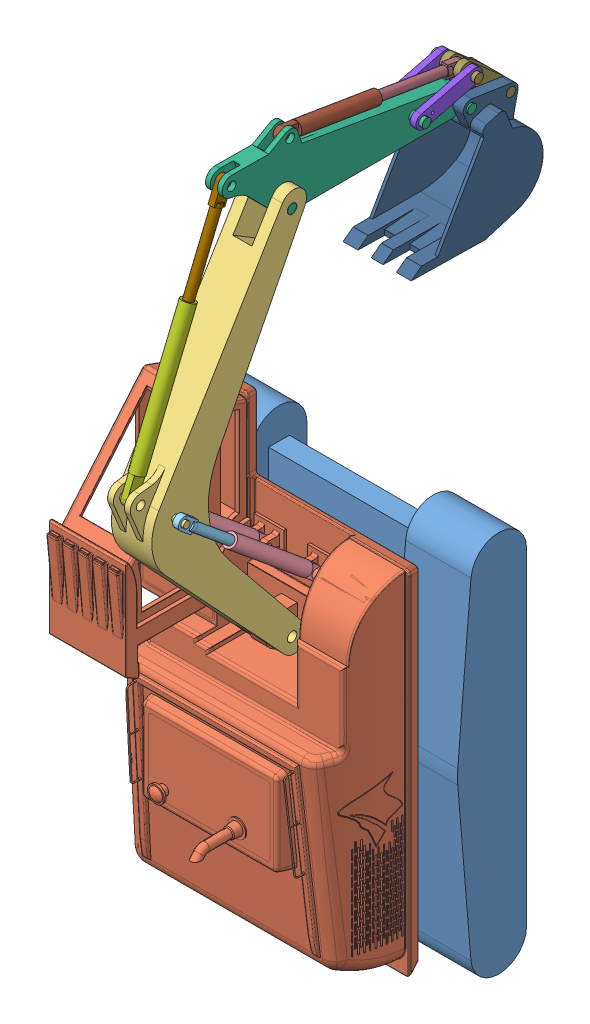
SolidWorks assembly MathScavator9000_flat, configuration Default. Lengths in mm.
Overall size (4800 11820.7 6568.15).
16 component instances, 13 part files, 33 mates.
Components (placement in the parent):
- ExcavatorBase-1: ExcavatorBase [Default] at origin size (4800 6440 1295)
- Chassis_Primary_v2_PART-1: Chassis_Primary_v2_PART [Default] at origin size (3985.01 7287.04 2544.86)
- Boom-2: Boom [Default] at (93.9527 -17.4087 507.5917) size (1080 6775.47 2834.12)
- BoomCyl-2: BoomCyl [Default] at (-446.0473 882.5913 372.5917) x (1 0 0) z (0 0.637047 0.770825) size (223.61 223.61 1900)
- BoomCyl-3: BoomCyl [Default] at (453.9527 882.5913 372.5917) x (1 0 0) z (0 0.637047 0.770825) size (223.61 223.61 1900)
- BoomPiston-2: BoomPiston [Default] at (453.9527 2698.8825 2570.2977) x (1 0 0) z (0 0.637047 0.770825) size (163.61 200 2150)
- BoomPiston-3: BoomPiston [Default] at (-446.0473 2698.8825 2570.2977) x (1 0 0) z (0 0.637047 0.770825) size (163.61 200 2150)
- Stick-1: Stick [Default] at (3.9527 6222.5913 597.5917) size (780 1210.11 4089.97)
- StickCyl-1: StickCyl [Default] at (5.9527 3022.5913 2997.5917) x (1 0 0) z (0 0.924264 -0.381754) size (223.61 223.61 2700)
- StickLink-1: StickLink [Default] at (259.9527 6362.5913 -1642.4083) x (1 0.000056 -0.000224) z (0 0.970634 0.240563) size (100.26 1142.82 240)
- StickLink-2: StickLink [Default] at (-252.0473 6362.5913 -1642.4083) x (1 0.000056 -0.000224) z (0 0.970634 0.240563) size (100.26 1142.82 240)
- StickPiston-1: StickPiston [Default] at (5.9527 6857.8328 1413.4982) x (1 0 0) z (0 0.924264 -0.381754) size (163.61 200 2500)
- Bucket-2: Bucket [Default] at (-1.2473 6213.4488 -2381.9895) size (1148 1959.94 2219.62)
- BucketCyl-2: BucketCyl [Default] at (3.9527 7066.1756 430.7297) x (1 0 0) z (0 -0.162718 -0.986673) size (223.61 223.61 1700)
- BucketLink-2: BucketLink [Default] at (1.9047 6579.7703 -2518.6916) x (1 0.000009 0.00001) z (-0.000013 0.657221 0.753698) size (738.41 251.24 966.87)
- BucketPiston-2: BucketPiston [Default] at (3.9527 6579.7703 -2518.6916) x (1 0 0) z (0 -0.162718 -0.986673) size (163.61 200 1600)
Mates (geometry in assembly coordinates):
- Concentric1: concentric aligned: cylinder of Chassis_Primary_v2_PART-1 through (138.9527 -17.4087 597.5917) axis (1 0 0) radius 80; cylinder of Boom-2 through (343.9527 -17.4087 597.5917) axis (1 0 0) radius 80
- Distance1: distance = 25 mm anti-aligned: plane of Boom-2 through (-156.0473 -1696.3395 2013.4684) normal (1 0 0); plane of Chassis_Primary_v2_PART-1 through (-131.0473 -17.4087 597.5917) normal (-1 0 0)
- Concentric2: concentric aligned: cylinder of Chassis_Primary_v2_PART-1 through (-621.0473 882.5913 372.5917) axis (-1 0 0) radius 40; cylinder of BoomCyl-2 through (-496.0473 882.5913 372.5917) axis (-1 0 0) radius 40
- Distance2: distance = 25 mm anti-aligned: plane of BoomCyl-2 through (-396.0473 959.6738 308.887) normal (1 0 0); plane of Chassis_Primary_v2_PART-1 through (-371.0473 882.5913 372.5917) normal (-1 0 0)
- Distance3: distance = 25 mm anti-aligned: plane of BoomCyl-3 through (403.9527 882.5913 372.5917) normal (-1 0 0); plane of Chassis_Primary_v2_PART-1 through (378.9527 882.5913 372.5917) normal (1 0 0)
- Concentric4: concentric anti-aligned: cylinder of Chassis_Primary_v2_PART-1 through (378.9527 882.5913 372.5917) axis (1 0 0) radius 40; cylinder of BoomCyl-3 through (403.9527 882.5913 372.5917) axis (-1 0 0) radius 40
- Concentric5: concentric anti-aligned: cylinder of Boom-2 through (343.9527 2698.8825 2570.2977) axis (1 0 0) radius 55; cylinder of BoomPiston-2 through (403.9527 2698.8825 2570.2977) axis (-1 0 0) radius 60
- Concentric6: concentric anti-aligned: cylinder of Boom-2 through (-536.0473 2698.8825 2570.2977) axis (1 0 0) radius 55; cylinder of BoomPiston-3 through (-496.0473 2698.8825 2570.2977) axis (-1 0 0) radius 60
- Concentric7: concentric aligned: cylinder of BoomCyl-3 through (453.9527 2029.2762 1760.0764) axis (0 0.637047 0.770825) radius 75; cylinder of BoomPiston-2 through (453.9527 1392.9358 990.1068) axis (0 0.637047 0.770825) radius 72.5
- Concentric8: concentric aligned: cylinder of BoomCyl-2 through (-446.0473 2029.2762 1760.0764) axis (0 0.637047 0.770825) radius 75; cylinder of BoomPiston-3 through (-446.0473 1392.9358 990.1068) axis (0 0.637047 0.770825) radius 72.5
- Concentric9: concentric aligned: cylinder of Boom-2 through (95.9527 3022.5913 2997.5917) axis (-1 0 0) radius 72; cylinder of StickCyl-1 through (-44.0473 3022.5913 2997.5917) axis (-1 0 0) radius 40
- Distance4: distance = 40 mm anti-aligned: plane of StickCyl-1 through (55.9527 3091.9111 2968.9601) normal (1 0 0); plane of Boom-2 through (95.9527 3022.5913 2997.5917) normal (-1 0 0)
- Concentric10: concentric aligned: cylinder of Boom-2 through (163.9527 6222.5913 597.5917) axis (-1 0 0) radius 80; cylinder of Stick-1 through (343.9527 6222.5913 597.5917) axis (-1 0 0) radius 75
- Distance5: distance = 20 mm anti-aligned: plane of Stick-1 through (143.9527 6222.5913 -2282.4083) normal (1 0 0); plane of Boom-2 through (163.9527 3864.7965 -2165.9151) normal (-1 0 0)
- Concentric11: concentric anti-aligned: cylinder of Stick-1 through (143.9527 6857.8328 1413.4982) axis (1 0 0) radius 72; cylinder of StickPiston-1 through (-44.0473 6857.8328 1413.4982) axis (-1 0 0) radius 60
- Concentric12: concentric aligned: cylinder of StickCyl-1 through (5.9527 5425.6772 2005.0303) axis (0 0.924264 -0.381754) radius 75; cylinder of StickPiston-1 through (5.9527 4639.5997 2329.7087) axis (0 0.924264 -0.381754) radius 72.5
- Concentric13: concentric aligned: cylinder of StickLink-1 through (209.9527 6362.5913 -1642.4083) axis (1 0 0) radius 75; cylinder of StickLink-2 through (-302.0473 6362.5913 -1642.4083) axis (1 0 0) radius 75
- Concentric14: concentric anti-aligned: cylinder of Stick-1 through (369.9527 6362.5913 -1642.4083) axis (-1 0 0) radius 75; cylinder of StickLink-2 through (-302.0473 6362.5913 -1642.4083) axis (1 0 0) radius 75
- Distance6: distance = 60 mm aligned: plane of Stick-1 through (-362.0473 6362.5913 -1642.4083) normal (-1 0 0); plane of StickLink-2 through (-302.0473 6579.7703 -2518.6916) normal (-1 0 0)
- Distance7: distance = 60 mm aligned: plane of Stick-1 through (369.9527 6362.5913 -1717.4083) normal (1 0 0); plane of StickLink-1 through (309.9527 6579.7703 -2518.6916) normal (1 0 0)
- Concentric15: concentric aligned: cylinder of StickLink-1 through (209.9527 6579.7703 -2518.6916) axis (1 0 0) radius 75; cylinder of StickLink-2 through (-302.0473 6579.7703 -2518.6916) axis (1 0 0) radius 75
- Concentric16: concentric anti-aligned: cylinder of Stick-1 through (143.9527 7066.1756 430.7297) axis (1 0 0) radius 72; cylinder of BucketCyl-2 through (-46.0473 7066.1756 430.7297) axis (-1 0 0) radius 40
- Distance8: distance = 10 mm anti-aligned: plane of BucketCyl-2 through (53.9527 7053.9717 356.7293) normal (1 0 0); plane of Stick-1 through (63.9527 6222.5913 -2282.4083) normal (-1 0 0)
- Concentric17: concentric aligned: cylinder of Bucket-2 through (192.9527 6109.4488 -3058.0535) axis (-1 0 0) radius 75; cylinder of BucketLink-2 through (372.9527 6109.4488 -3058.0535) axis (-1 0 0) radius 75
- Distance9: distance = 4 mm aligned: plane of BucketLink-2 through (372.9527 6171.1889 -3100.6347) normal (1 0 0); plane of Bucket-2 through (368.9527 6213.4488 -2381.9895) normal (1 0 0)
- Concentric18: concentric anti-aligned: cylinder of StickLink-1 through (209.9527 6579.7703 -2518.6916) axis (1 0 0) radius 75; cylinder of BucketLink-2 through (372.9527 6579.7703 -2518.6916) axis (-1 0 0) radius 75
- Concentric19: concentric anti-aligned: cylinder of Stick-1 through (143.9527 6213.4488 -2381.9895) axis (1 0 0) radius 75; cylinder of Bucket-2 through (192.9527 6213.4488 -2381.9895) axis (-1 0 0) radius 75
- Distance10: distance = 25 mm aligned: plane of Bucket-2 through (368.9527 6213.4488 -2381.9895) normal (1 0 0); plane of Stick-1 through (393.9527 6213.4488 -2381.9895) normal (1 0 0)
- Concentric20: concentric aligned: cylinder of BucketLink-2 through (63.7527 6579.7703 -2518.6916) axis (-1 0 0) radius 75; cylinder of BucketPiston-2 through (-46.0473 6579.7703 -2518.6916) axis (-1 0 0) radius 60
- Concentric21: concentric aligned: cylinder of BucketCyl-2 through (3.9527 6805.8274 -1147.9466) axis (0 -0.162718 -0.986673) radius 75; cylinder of BucketPiston-2 through (3.9527 6823.8467 -1038.6826) axis (0 -0.162718 -0.986673) radius 72.5
- Parallel19: parallel aligned: unknown of Boom-2
- Parallel20: parallel aligned: plane of Boom-2; plane of Stick-1
- Parallel21: parallel aligned: plane of Stick-1 through (3.9527 6222.5913 597.5917) normal (0 0 1); plane of Bucket-2 through (-1.2473 6213.4488 -2381.9895) normal (0 0 1)
